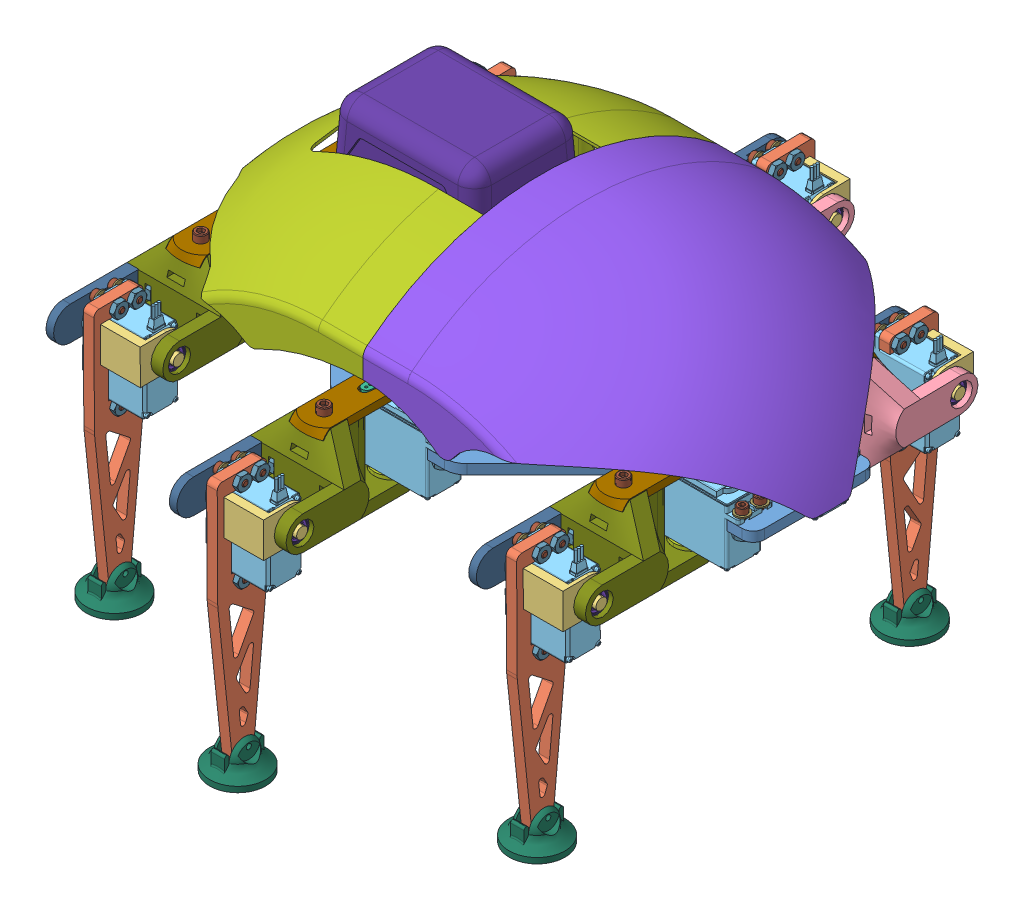
SolidWorks assembly Hexapod_NewBody, configuration Défaut. Lengths in mm. (continued)
Components (placement in the parent): (continued)
- Battery-1: Battery [Défaut] at (-118.1821 62.8376 15.5603) x (0 0 -1) z (-1 0 0) size (64.47 74.3 85.78)
  - MAKITA 4.0AH-1: MAKITA 4.0AH [Défaut] at (0.5853 -29.7874 85.4436) size (64.47 57.15 85.78)
  - MAKITA 4.0AH MOBILE-1: MAKITA 4.0AH MOBILE [Défaut] at (0.5853 -39.3124 91.7936) size (45.84 26.68 66.29)
- arduinoMega-1: arduinoMega [Detailed] at (-199.11 -7.6 14.62) x (0 0 -1) z (-1 0 0) size (108.32 14.5 53.3)
- raspberryPi3B-1: raspberryPi3B [Detailed] at (-109 6.35 15) x (-1 0 0) z (0 1 0) size (87.05 58.5 19.5)
- 12Channel PWM-1: 12Channel PWM [Default] at (-145.6 -5.6 15) x (-1 0 0) z (0 0 1) size (25.4 7.55 66.7)
- DROK_090483.stp-1: DROK_090483.stp [Default] at (-77.5 -5.6 45) x (-1 0 0) z (0 -1 0) size (50.02 60 18.9)
- socket head cap screw_ai-2: socket head cap screw_ai [HX-SHCS 0.138-32x0.625x0.625-N] at (-40.288 3.5052 19.09) x (0 -1 0) z (1 0 0) size (19.38 5.74 5.74)
- socket head cap screw_ai-3: socket head cap screw_ai [HX-SHCS 0.138-32x0.625x0.625-N] at (-50.288 3.5052 19.09) x (0 -1 0) z (0.5 0 0.866025) size (19.38 5.74 5.74)
- socket head cap screw_ai-4: socket head cap screw_ai [HX-SHCS 0.138-32x0.625x0.625-N] at (-50.288 3.5052 10.91) x (0 -1 0) z (1 0 0) size (19.38 5.74 5.74)
- socket head cap screw_ai-5: socket head cap screw_ai [HX-SHCS 0.138-32x0.625x0.625-N] at (-40.288 3.5052 10.91) x (0 -1 0) z (1 0 0) size (19.38 5.74 5.74)
- socket head cap screw_ai-6: socket head cap screw_ai [HX-SHCS 0.138-32x0.625x0.625-N] at (-170.288 3.5052 69.09) x (0 -1 0) z (1 0 0) size (19.38 5.74 5.74)
- socket head cap screw_ai-7: socket head cap screw_ai [HX-SHCS 0.138-32x0.625x0.625-N] at (-160.288 3.5052 69.09) x (0 -1 0) z (1 0 0) size (19.38 5.74 5.74)
- socket head cap screw_ai-14: socket head cap screw_ai [HX-SHCS 0.138-32x0.625x0.625-N] at (-160.288 3.5052 -39.09) x (0 -1 0) z (1 0 0) size (19.38 5.74 5.74)
- socket head cap screw_ai-15: socket head cap screw_ai [HX-SHCS 0.138-32x0.625x0.625-N] at (-170.288 3.5052 -39.09) x (0 -1 0) z (1 0 0) size (19.38 5.74 5.74)
- socket head cap screw_ai-16: socket head cap screw_ai [HX-SHCS 0.138-32x0.625x0.625-N] at (-280.288 3.5052 19.09) x (0 -1 0) z (1 0 0) size (19.38 5.74 5.74)
- socket head cap screw_ai-17: socket head cap screw_ai [HX-SHCS 0.138-32x0.625x0.625-N] at (-290.288 3.5052 19.09) x (0 -1 0) z (0.5 0 0.866025) size (19.38 5.74 5.74)
- socket head cap screw_ai-18: socket head cap screw_ai [HX-SHCS 0.138-32x0.625x0.625-N] at (-290.288 3.5052 10.91) x (0 -1 0) z (1 0 0) size (19.38 5.74 5.74)
- socket head cap screw_ai-19: socket head cap screw_ai [HX-SHCS 0.138-32x0.625x0.625-N] at (-280.288 3.5052 10.91) x (0 -1 0) z (1 0 0) size (19.38 5.74 5.74)
- machine screw nut hex_ai-60: machine screw nut hex_ai [MSHXNUT 0.138-32-D-N] at (-298.75 -8.4956 -15.08) x (1 0 0) z (0 -1 0) size (7.92 9.15 2.9)
- machine screw nut hex_ai-65: machine screw nut hex_ai [MSHXNUT 0.138-32-D-N] at (-298.75 -8.4956 -4.92) x (1 0 0) z (0 -1 0) size (7.92 9.15 2.9)
- machine screw nut hex_ai-70: machine screw nut hex_ai [MSHXNUT 0.138-32-D-N] at (-251.252 -8.4956 -4.92) x (0.5 0 0.866025) z (0 -1 0) size (7.92 9.15 2.9)
- machine screw nut hex_ai-75: machine screw nut hex_ai [MSHXNUT 0.138-32-D-N] at (-251.252 -8.4956 -15.08) x (0.5 0 0.866025) z (0 -1 0) size (7.92 9.15 2.9)
- machine screw nut hex_ai-80: machine screw nut hex_ai [MSHXNUT 0.138-32-D-N] at (-280.288 -13.5656 10.91) x (0 0 1) z (0 -1 0) size (7.92 9.15 2.9)
- machine screw nut hex_ai-85: machine screw nut hex_ai [MSHXNUT 0.138-32-D-N] at (-290.288 -13.5656 10.91) x (0 0 1) z (0 -1 0) size (7.92 9.15 2.9)
- machine screw nut hex_ai-63: machine screw nut hex_ai [MSHXNUT 0.138-32-D-N] at (-178.75 -8.4956 -65.08) x (1 0 0) z (0 -1 0) size (7.92 9.15 2.9)
- machine screw nut hex_ai-68: machine screw nut hex_ai [MSHXNUT 0.138-32-D-N] at (-178.75 -8.4956 -54.92) x (1 0 0) z (0 -1 0) size (7.92 9.15 2.9)
- machine screw nut hex_ai-73: machine screw nut hex_ai [MSHXNUT 0.138-32-D-N] at (-131.252 -8.4956 -54.92) x (0.5 0 0.866025) z (0 -1 0) size (7.92 9.15 2.9)
- machine screw nut hex_ai-78: machine screw nut hex_ai [MSHXNUT 0.138-32-D-N] at (-131.252 -8.4956 -65.08) x (0.5 0 0.866025) z (0 -1 0) size (7.92 9.15 2.9)
- machine screw nut hex_ai-83: machine screw nut hex_ai [MSHXNUT 0.138-32-D-N] at (-160.288 -13.5656 -39.09) x (0 0 1) z (0 -1 0) size (7.92 9.15 2.9)
- machine screw nut hex_ai-86: machine screw nut hex_ai [MSHXNUT 0.138-32-D-N] at (-170.288 -13.5656 -39.09) x (0 0 1) z (0 -1 0) size (7.92 9.15 2.9)
- machine screw nut hex_ai-87: machine screw nut hex_ai [MSHXNUT 0.138-32-D-N] at (-50.288 -13.5656 10.91) x (0 0 1) z (0 -1 0) size (7.92 9.15 2.9)
- machine screw nut hex_ai-84: machine screw nut hex_ai [MSHXNUT 0.138-32-D-N] at (-40.288 -13.5656 10.91) x (0 0 1) z (0 -1 0) size (7.92 9.15 2.9)
- machine screw nut hex_ai-74: machine screw nut hex_ai [MSHXNUT 0.138-32-D-N] at (-11.252 -8.4956 -4.92) x (0.5 0 0.866025) z (0 -1 0) size (7.92 9.15 2.9)
- machine screw nut hex_ai-79: machine screw nut hex_ai [MSHXNUT 0.138-32-D-N] at (-11.252 -8.4956 -15.08) x (0.5 0 0.866025) z (0 -1 0) size (7.92 9.15 2.9)
- machine screw nut hex_ai-69: machine screw nut hex_ai [MSHXNUT 0.138-32-D-N] at (-58.75 -8.4956 -4.92) x (1 0 0) z (0 -1 0) size (7.92 9.15 2.9)
- machine screw nut hex_ai-64: machine screw nut hex_ai [MSHXNUT 0.138-32-D-N] at (-58.75 -8.4956 -15.08) x (1 0 0) z (0 -1 0) size (7.92 9.15 2.9)
- machine screw nut hex_ai-88: machine screw nut hex_ai [MSHXNUT 0.138-32-D-N] at (-290.288 -10.67 19.09) x (0 0 -1) z (0 1 0) size (7.92 9.15 2.9)
- machine screw nut hex_ai-89: machine screw nut hex_ai [MSHXNUT 0.138-32-D-N] at (-280.288 -10.67 19.09) x (0 0 -1) z (0 1 0) size (7.92 9.15 2.9)
- machine screw nut hex_ai-90: machine screw nut hex_ai [MSHXNUT 0.138-32-D-N] at (-251.252 -5.6 34.92) x (0.5 0 -0.866025) z (0 1 0) size (7.92 9.15 2.9)
- machine screw nut hex_ai-91: machine screw nut hex_ai [MSHXNUT 0.138-32-D-N] at (-251.252 -5.6 45.08) x (0.5 0 -0.866025) z (0 1 0) size (7.92 9.15 2.9)
- machine screw nut hex_ai-92: machine screw nut hex_ai [MSHXNUT 0.138-32-D-N] at (-298.75 -5.6 34.92) x (1 0 0) z (0 1 0) size (7.92 9.15 2.9)
- machine screw nut hex_ai-93: machine screw nut hex_ai [MSHXNUT 0.138-32-D-N] at (-298.75 -5.6 45.08) x (1 0 0) z (0 1 0) size (7.92 9.15 2.9)
- machine screw nut hex_ai-94: machine screw nut hex_ai [MSHXNUT 0.138-32-D-N] at (-178.75 -5.6 95.08) x (1 0 0) z (0 1 0) size (7.92 9.15 2.9)
- machine screw nut hex_ai-95: machine screw nut hex_ai [MSHXNUT 0.138-32-D-N] at (-178.75 -5.6 84.92) x (1 0 0) z (0 1 0) size (7.92 9.15 2.9)
- machine screw nut hex_ai-96: machine screw nut hex_ai [MSHXNUT 0.138-32-D-N] at (-131.252 -5.6 84.92) x (0.5 0 -0.866025) z (0 1 0) size (7.92 9.15 2.9)
- machine screw nut hex_ai-97: machine screw nut hex_ai [MSHXNUT 0.138-32-D-N] at (-131.252 -5.6 95.08) x (0.5 0 -0.866025) z (0 1 0) size (7.92 9.15 2.9)
- machine screw nut hex_ai-98: machine screw nut hex_ai [MSHXNUT 0.138-32-D-N] at (-160.288 -10.67 69.09) x (0 0 -1) z (0 1 0) size (7.92 9.15 2.9)
- machine screw nut hex_ai-99: machine screw nut hex_ai [MSHXNUT 0.138-32-D-N] at (-170.288 -10.67 69.09) x (0 0 -1) z (0 1 0) size (7.92 9.15 2.9)
- machine screw nut hex_ai-100: machine screw nut hex_ai [MSHXNUT 0.138-32-D-N] at (-50.288 -10.67 19.09) x (0 0 -1) z (0 1 0) size (7.92 9.15 2.9)
- machine screw nut hex_ai-101: machine screw nut hex_ai [MSHXNUT 0.138-32-D-N] at (-40.288 -10.67 19.09) x (0 0 -1) z (0 1 0) size (7.92 9.15 2.9)
- machine screw nut hex_ai-102: machine screw nut hex_ai [MSHXNUT 0.138-32-D-N] at (-11.252 -5.6 34.92) x (0.5 0 -0.866025) z (0 1 0) size (7.92 9.15 2.9)
- machine screw nut hex_ai-103: machine screw nut hex_ai [MSHXNUT 0.138-32-D-N] at (-11.252 -5.6 45.08) x (0.5 0 -0.866025) z (0 1 0) size (7.92 9.15 2.9)
- machine screw nut hex_ai-104: machine screw nut hex_ai [MSHXNUT 0.138-32-D-N] at (-58.75 -5.6 34.92) x (1 0 0) z (0 1 0) size (7.92 9.15 2.9)
- machine screw nut hex_ai-105: machine screw nut hex_ai [MSHXNUT 0.138-32-D-N] at (-58.75 -5.6 45.08) x (1 0 0) z (0 1 0) size (7.92 9.15 2.9)
- socket head cap screw_ai-20: socket head cap screw_ai [HX-SHCS 0.138-32x0.5x0.5-N] at (-175 -12.6052 48.88) x (0 1 0) z (-0.5 0 -0.866025) size (16.21 5.74 5.74)
- socket head cap screw_ai-21: socket head cap screw_ai [HX-SHCS 0.138-32x0.5x0.5-N] at (-223.22 -12.6052 -32.36) x (0 1 0) z (1 0 0) size (16.21 5.74 5.74)
- socket head cap screw_ai-22: socket head cap screw_ai [HX-SHCS 0.138-32x0.5x0.5-N] at (-175 -12.6052 -26) x (0 1 0) z (-0.5 0 -0.866025) size (16.21 5.74 5.74)
- socket head cap screw_ai-23: socket head cap screw_ai [HX-SHCS 0.138-32x0.5x0.5-N] at (-223.22 -12.6052 50.11) x (0 1 0) z (-1 0 0) size (16.21 5.74 5.74)
- machine screw nut hex_ai-106: machine screw nut hex_ai [MSHXNUT 0.112-40-D-N] at (-223.22 2.4892 -32.36) x (1 0 0) z (0 1 0) size (6.35 7.33 2.49)
- machine screw nut hex_ai-107: machine screw nut hex_ai [MSHXNUT 0.112-40-D-N] at (-223.22 2.4892 50.11) x (1 0 0) z (0 1 0) size (6.35 7.33 2.49)
- machine screw nut hex_ai-108: machine screw nut hex_ai [MSHXNUT 0.112-40-D-N] at (-175 2.4892 -26) x (1 0 0) z (0 1 0) size (6.35 7.33 2.49)
- machine screw nut hex_ai-109: machine screw nut hex_ai [MSHXNUT 0.112-40-D-N] at (-175 2.4892 48.88) x (1 0 0) z (0 1 0) size (6.35 7.33 2.49)
- socket head cap screw_ai-24: socket head cap screw_ai [HX-SHCS 0.138-32x0.5x0.5-N] at (-117.315 -10.3052 -11.415) x (0 1 0) z (-0.5 0 -0.866025) size (16.21 5.74 5.74)
- machine screw nut hex_ai-110: machine screw nut hex_ai [MSHXNUT 0.112-40-D-N] at (-117.315 2.4892 -11.415) x (1 0 0) z (0 1 0) size (6.35 7.33 2.49)
- socket head cap screw_ai-25: socket head cap screw_ai [HX-SHCS 0.138-32x0.5x0.5-N] at (-80.685 -10.3052 -11.415) x (0 1 0) z (-0.5 0 -0.866025) size (16.21 5.74 5.74)
- socket head cap screw_ai-26: socket head cap screw_ai [HX-SHCS 0.138-32x0.5x0.5-N] at (-117.315 -10.3052 41.415) x (0 1 0) z (-0.5 0 -0.866025) size (16.21 5.74 5.74)
- socket head cap screw_ai-27: socket head cap screw_ai [HX-SHCS 0.138-32x0.5x0.5-N] at (-80.685 -10.3052 41.415) x (0 1 0) z (-0.5 0 -0.866025) size (16.21 5.74 5.74)
- machine screw nut hex_ai-111: machine screw nut hex_ai [MSHXNUT 0.112-40-D-N] at (-80.685 2.4892 -11.415) x (1 0 0) z (0 1 0) size (6.35 7.33 2.49)
- machine screw nut hex_ai-112: machine screw nut hex_ai [MSHXNUT 0.112-40-D-N] at (-117.315 2.4892 41.415) x (1 0 0) z (0 1 0) size (6.35 7.33 2.49)
- machine screw nut hex_ai-113: machine screw nut hex_ai [MSHXNUT 0.112-40-D-N] at (-80.685 2.4892 41.415) x (1 0 0) z (0 1 0) size (6.35 7.33 2.49)
- 1_4_Round_Aluminum_Standoff.step-1: 1_4_Round_Aluminum_Standoff.step [Défaut] at (-70 0 -9.5) x (0.963282 0 -0.268492) z (0.268492 0 0.963282) size (6.34 6.36 6.34)
- socket head cap screw_ai-28: socket head cap screw_ai [HX-SHCS 0.112-40x1x0.75-N] at (-70 10.4948 -9.5) x (0 -1 0) z (0.637638 0 0.770336) size (28.24 4.65 4.65)
- machine screw nut hex_ai-114: machine screw nut hex_ai [MSHXNUT 0.112-40-D-N] at (-70 -8.0892 -9.5) x (1 0 0) z (0 -1 0) size (6.35 7.33 2.49)
- 1_4_Round_Aluminum_Standoff.step-2: 1_4_Round_Aluminum_Standoff.step [Défaut] at (-128 0 -9.5) x (0.963282 0 -0.268492) z (0.268492 0 0.963282) size (6.34 6.36 6.34)
- 1_4_Round_Aluminum_Standoff.step-3: 1_4_Round_Aluminum_Standoff.step [Défaut] at (-70 0 39.5) x (0.963282 0 -0.268492) z (0.268492 0 0.963282) size (6.34 6.36 6.34)
- 1_4_Round_Aluminum_Standoff.step-4: 1_4_Round_Aluminum_Standoff.step [Défaut] at (-128 0 39.5) x (0.963282 0 -0.268492) z (0.268492 0 0.963282) size (6.34 6.36 6.34)
- machine screw nut hex_ai-115: machine screw nut hex_ai [MSHXNUT 0.112-40-D-N] at (-128 -8.0892 -9.5) x (1 0 0) z (0 -1 0) size (6.35 7.33 2.49)
- machine screw nut hex_ai-116: machine screw nut hex_ai [MSHXNUT 0.112-40-D-N] at (-70 -8.0892 39.5) x (1 0 0) z (0 -1 0) size (6.35 7.33 2.49)
- machine screw nut hex_ai-117: machine screw nut hex_ai [MSHXNUT 0.112-40-D-N] at (-128 -8.0892 39.5) x (1 0 0) z (0 -1 0) size (6.35 7.33 2.49)
- socket head cap screw_ai-29: socket head cap screw_ai [HX-SHCS 0.112-40x1x0.75-N] at (-128 10.4948 -9.5) x (0 -1 0) z (0.637638 0 0.770336) size (28.24 4.65 4.65)
- socket head cap screw_ai-30: socket head cap screw_ai [HX-SHCS 0.112-40x1x0.75-N] at (-70 10.4948 39.5) x (0 -1 0) z (0.637638 0 0.770336) size (28.24 4.65 4.65)
- socket head cap screw_ai-31: socket head cap screw_ai [HX-SHCS 0.112-40x1x0.75-N] at (-128 10.4948 39.5) x (0 -1 0) z (0.637638 0 0.770336) size (28.24 4.65 4.65)
- socket head cap screw_ai-32: socket head cap screw_ai [HX-SHCS 0.112-40x0.5x0.5-N] at (-155 -9.9448 -12.95) x (0 1 0) z (-1 0 0) size (15.54 4.65 4.65)
- machine screw nut hex_ai-118: machine screw nut hex_ai [MSHXNUT 0.112-40-D-N] at (-155 2.4892 -12.95) x (1 0 0) z (0 1 0) size (6.35 7.33 2.49)
- socket head cap screw_ai-33: socket head cap screw_ai [HX-SHCS 0.112-40x0.5x0.5-N] at (-136.2 -9.9448 -12.95) x (0 1 0) z (-1 0 0) size (15.54 4.65 4.65)
- socket head cap screw_ai-34: socket head cap screw_ai [HX-SHCS 0.112-40x0.5x0.5-N] at (-155 -9.9448 42.95) x (0 1 0) z (-1 0 0) size (15.54 4.65 4.65)
- socket head cap screw_ai-35: socket head cap screw_ai [HX-SHCS 0.112-40x0.5x0.5-N] at (-136.2 -9.9448 42.95) x (0 1 0) z (-1 0 0) size (15.54 4.65 4.65)
- machine screw nut hex_ai-119: machine screw nut hex_ai [MSHXNUT 0.112-40-D-N] at (-136.2 2.4892 -12.95) x (1 0 0) z (0 1 0) size (6.35 7.33 2.49)
- machine screw nut hex_ai-120: machine screw nut hex_ai [MSHXNUT 0.112-40-D-N] at (-155 2.4892 42.95) x (1 0 0) z (0 1 0) size (6.35 7.33 2.49)
- machine screw nut hex_ai-121: machine screw nut hex_ai [MSHXNUT 0.112-40-D-N] at (-136.2 2.4892 42.95) x (1 0 0) z (0 1 0) size (6.35 7.33 2.49)
- 1_4_Round_Aluminum_Standoff.step-5: 1_4_Round_Aluminum_Standoff.step [Défaut] at (-174 0 -7) x (0.963282 0 -0.268492) z (0.268492 0 0.963282) size (6.34 6.36 6.34)
- 1_4_Round_Aluminum_Standoff.step-6: 1_4_Round_Aluminum_Standoff.step [Défaut] at (-174 0 37) x (0.963282 0 -0.268492) z (0.268492 0 0.963282) size (6.34 6.36 6.34)
- 1_4_Round_Aluminum_Standoff.step-7: 1_4_Round_Aluminum_Standoff.step [Défaut] at (-240 0 -7) x (0.963282 0 -0.268492) z (0.268492 0 0.963282) size (6.34 6.36 6.34)
- 1_4_Round_Aluminum_Standoff.step-8: 1_4_Round_Aluminum_Standoff.step [Défaut] at (-240 0 37) x (0.963282 0 -0.268492) z (0.268492 0 0.963282) size (6.34 6.36 6.34)
- socket head cap screw_ai-40: socket head cap screw_ai [HX-SHCS 0.112-40x1x0.75-N] at (-174 -8.4448 -7) x (0 1 0) z (-0.415316 0 -0.909677) size (28.24 4.65 4.65)
- socket head cap screw_ai-41: socket head cap screw_ai [HX-SHCS 0.112-40x1x0.75-N] at (-174 -8.4448 37) x (0 1 0) z (-0.415316 0 -0.909677) size (28.24 4.65 4.65)
- socket head cap screw_ai-42: socket head cap screw_ai [HX-SHCS 0.112-40x1x0.75-N] at (-240 -8.4448 -7) x (0 1 0) z (-0.415316 0 -0.909677) size (28.24 4.65 4.65)
- socket head cap screw_ai-43: socket head cap screw_ai [HX-SHCS 0.112-40x1x0.75-N] at (-240 -8.4448 37) x (0 1 0) z (-0.415316 0 -0.909677) size (28.24 4.65 4.65)
- Batterie_holder-1: Batterie_holder [Default] at (-223 17.7 15) size (72 19.6 50)
- machine screw nut hex_ai-122: machine screw nut hex_ai [MSHXNUT 0.112-40-D-N] at (-174 15.1892 -7) x (1 0 0) z (0 1 0) size (6.35 7.33 2.49)
- machine screw nut hex_ai-123: machine screw nut hex_ai [MSHXNUT 0.112-40-D-N] at (-174 15.1892 37) x (1 0 0) z (0 1 0) size (6.35 7.33 2.49)
- machine screw nut hex_ai-124: machine screw nut hex_ai [MSHXNUT 0.112-40-D-N] at (-240 15.1892 -7) x (1 0 0) z (0 1 0) size (6.35 7.33 2.49)
- machine screw nut hex_ai-125: machine screw nut hex_ai [MSHXNUT 0.112-40-D-N] at (-240 15.1892 37) x (1 0 0) z (0 1 0) size (6.35 7.33 2.49)
- Shell_front-3: Shell_front [Default] at (-155 -76.2 15) x (0 0 1) z (-1 0 0) size (204.71 79.03 165.14)
- Shell_back-3: Shell_back [Default] at (-155 -76.2 15) x (0 0 -1) z (1 0 0) size (205.09 91.22 173.55)
Mates (geometry in assembly coordinates):
- Coincident2: coincident anti-aligned: plane of Body_V2-5 through (-295 -5.601 0) normal (0 0 -1)
- Coincident3: coincident aligned: plane of Body_V2-5 through (-310 0 15) normal (0 1 0)
- Coincident4: coincident aligned: plane of Body_V2-5 through (0 0 50) normal (1 0 0)
- Coincident5: coincident anti-aligned: plane of Body_V2-5 through (-310 0 15) normal (0 1 0); plane of Leg-6/hs-422-3 through (-35.001 0 -0.094) normal (0 -1 0)
- Concentric3: concentric anti-aligned: cylinder of Body_V2-5 through (-58.75 0 -15.08) axis (0 -1 0) radius 1.45; cylinder of Leg-6/hs-422-3 through (-58.75 -26.67 -15.08) axis (0 1 0) radius 2.1844
- Concentric6: concentric aligned: cylinder of Body_V2-5 through (-298.75 -5.601 -4.92) axis (0 1 0) radius 1.45; cylinder of Leg-7/hs-422-3 through (-298.75 -26.67 -4.92) axis (0 1 0) radius 2.1844
- Parallel4: parallel anti-aligned: plane of Body_V2-5 through (-295 -5.601 0) normal (0 0 -1); plane of Leg-7/hs-422-3 through (-275.001 -5.969 -0.094) normal (0 0 1)
- Coincident9: coincident anti-aligned: plane of Body_V2-5 through (-310 0 15) normal (0 1 0); plane of Leg-7/hs-422-3 through (-275.001 0 -0.094) normal (0 -1 0)
- Coincident10: coincident anti-aligned: plane of Body_V2-5 through (-310 0 15) normal (0 1 0); plane of Leg-8/hs-422-3 through (-155.001 0 -50.094) normal (0 -1 0)
- Concentric7: concentric anti-aligned: cylinder of Body_V2-5 through (-178.75 0 -54.92) axis (0 -1 0) radius 1.45; cylinder of Leg-8/hs-422-3 through (-178.75 -26.67 -54.92) axis (0 1 0) radius 2.1844
- Parallel5: parallel anti-aligned: plane of Body_V2-5 through (-175 -5.6 -50) normal (0 0 -1); plane of Leg-8/hs-422-3 through (-155.001 -5.969 -50.094) normal (0 0 1)
- Parallel6: parallel anti-aligned: plane of Body_V2-5 through (-55 -5.6 0) normal (0 0 -1); plane of Leg-6/hs-422-3 through (-35.001 -5.969 -0.094) normal (0 0 1)
- Coincident11: coincident anti-aligned: plane of Body_V2-5 through (-310 0 15) normal (0 1 0); plane of Leg_(Straight_Foot)_(Mirror)-4/hs-422-3 through (-275.001 0 49.906) normal (0 -1 0)
- Concentric8: concentric aligned: cylinder of Body_V2-5 through (-298.75 -5.601 45.08) axis (0 1 0) radius 1.45; cylinder of Leg_(Straight_Foot)_(Mirror)-4/hs-422-3 through (-298.75 -26.67 45.08) axis (0 1 0) radius 2.1844
- Parallel7: parallel anti-aligned: plane of Body_V2-5 through (-295 -5.601 30) normal (0 0 1); plane of Leg_(Straight_Foot)_(Mirror)-4/hs-422-3 through (-275.001 -5.969 30.094) normal (0 0 -1)
- Coincident13: coincident anti-aligned: plane of Body_V2-5 through (-310 0 15) normal (0 1 0); plane of Leg_(Straight_Foot)_(Mirror)-5/hs-422-3 through (-35.001 0 49.906) normal (0 -1 0)
- Concentric9: concentric anti-aligned: cylinder of Body_V2-5 through (-58.75 0 45.08) axis (0 -1 0) radius 1.45; cylinder of Leg_(Straight_Foot)_(Mirror)-5/hs-422-3 through (-58.75 -26.67 45.08) axis (0 1 0) radius 2.1844
- Parallel8: parallel anti-aligned: plane of Body_V2-5 through (-55 -5.6 30) normal (0 0 1); plane of Leg_(Straight_Foot)_(Mirror)-5/hs-422-3 through (-35.001 -5.969 30.094) normal (0 0 -1)
- Coincident15: coincident anti-aligned: plane of Body_V2-5 through (-310 0 15) normal (0 1 0); plane of Leg_(Straight_Foot)_(Mirror)-6/hs-422-3 through (-155.001 0 99.906) normal (0 -1 0)
- Concentric10: concentric anti-aligned: cylinder of Body_V2-5 through (-178.75 0 95.08) axis (0 -1 0) radius 1.45; cylinder of Leg_(Straight_Foot)_(Mirror)-6/hs-422-3 through (-178.75 -26.67 95.08) axis (0 1 0) radius 2.1844
- Parallel9: parallel anti-aligned: plane of Body_V2-5 through (-175 -5.6 80) normal (0 0 1); plane of Leg_(Straight_Foot)_(Mirror)-6/hs-422-3 through (-155.001 -5.969 80.094) normal (0 0 -1)
- Coïncidente2: coincident anti-aligned: plane of arduinoMega-1 through (-199.11 -5.6 14.62) normal (0 1 0); plane of Body_V2-5 through (-310 -5.6 15) normal (0 -1 0)
- Coïncidente4: coincident anti-aligned: plane of Body_V2-5 through (-310 -5.6 15) normal (0 -1 0); plane of 12Channel PWM-1 through (-155 -5.6 -12.95) normal (0 1 0)
- Coïncidente5: coincident anti-aligned: plane of Body_V2-5 through (-310 -5.6 15) normal (0 -1 0); plane of DROK_090483.stp-1 through (-99 -5.6 15) normal (0 1 0)
- Parallèle4: parallel aligned: plane of Body_V2-5 through (0 0 50) normal (1 0 0); plane of 12Channel PWM-1 through (-132.9 -7.1 -12.95) normal (1 0 0)
- Concentric13: concentric aligned: cylinder of Body_V2-5 through (-155 0 42.95) axis (0 -1 0) radius 1.25; cylinder of 12Channel PWM-1 through (-155 -2.0645 42.95) axis (0 -1 0) radius 1.25
- Concentric17: concentric anti-aligned: circle of Body-1; circle of DROK_090483.stp-1
- Concentric18: concentric aligned: cylinder of Body_V2-5 through (-80.685 0 41.415) axis (0 -1 0) radius 1.45; cylinder of DROK_090483.stp-1 through (-80.685 -5.6 41.415) axis (0 -1 0) radius 1.585
- Concentric19: concentric aligned: cylinder of Body_V2-5 through (-175 0 -26) axis (0 -1 0) radius 1.6; circle of arduinoMega-1
- Concentric22: concentric aligned: cylinder of Body_V2-5 through (-223.22 0 50.11) axis (0 -1 0) radius 1.6; cylinder of arduinoMega-1 through (-223.22 -7.6 50.11) axis (0 -1 0) radius 1.6
- Concentric23: concentric anti-aligned: cylinder of Body_V2-5 through (-40.288 0 19.09) axis (0 -1 0) radius 1.45; cylinder of socket head cap screw_ai-2 through (-40.288 35.2552 19.09) axis (0 1 0) radius 1.7526
- Concentric24: concentric anti-aligned: cylinder of Body_V2-5 through (-50.288 0 19.09) axis (0 -1 0) radius 1.45; cylinder of socket head cap screw_ai-3 through (-50.288 35.2552 19.09) axis (0 1 0) radius 1.7526
- Coincident19: coincident anti-aligned: plane of Body_V2-5 through (-310 0 15) normal (0 1 0); plane of socket head cap screw_ai-2 through (-40.288 0 16.2198) normal (0 -1 0)
- Coincident20: coincident anti-aligned: plane of Body_V2-5 through (-310 0 15) normal (0 1 0); plane of socket head cap screw_ai-3 through (-47.8023 0 17.6549) normal (0 -1 0)
- Parallel10: parallel aligned: plane of Body_V2-5 through (0 0 50) normal (1 0 0); plane of socket head cap screw_ai-3 through (-51.6723 1.8796 19.8892) normal (1 0 0)
- Parallel11: parallel aligned: plane of Body_V2-5 through (0 0 50) normal (1 0 0); plane of socket head cap screw_ai-2 through (-41.6723 1.8796 18.2908) normal (1 0 0)
- Concentric25: concentric anti-aligned: cylinder of Body_V2-5 through (-50.288 0 10.91) axis (0 -1 0) radius 1.45; cylinder of socket head cap screw_ai-4 through (-50.288 35.2552 10.91) axis (0 1 0) radius 1.7526
- Concentric26: concentric anti-aligned: cylinder of Body_V2-5 through (-40.288 0 10.91) axis (0 -1 0) radius 1.45; cylinder of socket head cap screw_ai-5 through (-40.288 35.2552 10.91) axis (0 1 0) radius 1.7526
- Coincident23: coincident anti-aligned: plane of Body_V2-5 through (-310 0 15) normal (0 1 0); plane of socket head cap screw_ai-5 through (-40.288 0 8.0398) normal (0 -1 0)
- Coincident24: coincident anti-aligned: plane of Body_V2-5 through (-310 0 15) normal (0 1 0); plane of socket head cap screw_ai-4 through (-50.288 0 8.0398) normal (0 -1 0)
- Parallel12: parallel aligned: plane of Body_V2-5 through (0 0 50) normal (1 0 0); plane of socket head cap screw_ai-5 through (-41.6723 1.8796 10.1108) normal (1 0 0)
- Parallel13: parallel aligned: plane of Body_V2-5 through (0 0 50) normal (1 0 0); plane of socket head cap screw_ai-4 through (-51.6723 1.8796 10.1108) normal (1 0 0)
- Concentric27: concentric anti-aligned: cylinder of Body_V2-5 through (-170.288 0 -39.09) axis (0 -1 0) radius 1.45; cylinder of HX-SHCS 0.138-32x0.625x0.625-N-13 through (-214.94 40.2807 -39.09) axis (0 1 0) radius 1.7526
- Concentric29: concentric anti-aligned: cylinder of Body_V2-5 through (-160.288 0 69.09) axis (0 -1 0) radius 1.45; cylinder of socket head cap screw_ai-7 through (-160.288 35.2552 69.09) axis (0 1 0) radius 1.7526
- Concentric30: concentric anti-aligned: cylinder of Body_V2-5 through (-170.288 0 69.09) axis (0 -1 0) radius 1.45; cylinder of socket head cap screw_ai-6 through (-170.288 35.2552 69.09) axis (0 1 0) radius 1.7526
- Coincident27: coincident anti-aligned: plane of Body_V2-5 through (-310 0 15) normal (0 1 0); plane of socket head cap screw_ai-7 through (-160.288 0 66.2198) normal (0 -1 0)
- Coincident28: coincident anti-aligned: plane of Body_V2-5 through (-310 0 15) normal (0 1 0); plane of socket head cap screw_ai-6 through (-170.288 0 66.2198) normal (0 -1 0)
- Parallel14: parallel aligned: plane of Body_V2-5 through (0 0 50) normal (1 0 0); plane of socket head cap screw_ai-6 through (-171.6723 1.8796 68.2908) normal (1 0 0)
- Parallel15: parallel aligned: plane of Body_V2-5 through (0 0 50) normal (1 0 0); plane of socket head cap screw_ai-7 through (-161.6723 1.8796 68.2908) normal (1 0 0)
- Concentric31: concentric anti-aligned: cylinder of Body_V2-5 through (-170.288 0 -39.09) axis (0 -1 0) radius 1.45; cylinder of socket head cap screw_ai-15 through (-170.288 35.2552 -39.09) axis (0 1 0) radius 1.7526
- Concentric32: concentric anti-aligned: cylinder of Body_V2-5 through (-160.288 0 -39.09) axis (0 -1 0) radius 1.45; cylinder of socket head cap screw_ai-14 through (-160.288 35.2552 -39.09) axis (0 1 0) radius 1.7526
- Coincident31: coincident anti-aligned: plane of Body_V2-5 through (-310 0 15) normal (0 1 0); plane of socket head cap screw_ai-15 through (-170.288 0 -41.9602) normal (0 -1 0)
- Coincident32: coincident anti-aligned: plane of Body_V2-5 through (-310 0 15) normal (0 1 0); plane of socket head cap screw_ai-14 through (-160.288 0 -41.9602) normal (0 -1 0)
- Parallel16: parallel anti-aligned: plane of Body_V2-5 through (0 0 50) normal (1 0 0); plane of socket head cap screw_ai-15 through (-168.9037 1.8796 -38.2908) normal (-1 0 0)
- Parallel17: parallel anti-aligned: plane of Body_V2-5 through (0 0 50) normal (1 0 0); plane of socket head cap screw_ai-14 through (-158.9037 1.8796 -38.2908) normal (-1 0 0)
- Concentric33: concentric aligned: cylinder of Body_V2-5 through (-290.288 -5.601 19.09) axis (0 1 0) radius 1.45; cylinder of socket head cap screw_ai-17 through (-290.288 35.2552 19.09) axis (0 1 0) radius 1.7526
- Concentric34: concentric aligned: circle of Body-1; cylinder of socket head cap screw_ai-16 through (-280.288 35.2552 19.09) axis (0 1 0) radius 1.7526
- Concentric35: concentric aligned: cylinder of Body_V2-5 through (-290.288 -5.601 10.91) axis (0 1 0) radius 1.45; cylinder of socket head cap screw_ai-18 through (-290.288 35.2552 10.91) axis (0 1 0) radius 1.7526
- Concentric36: concentric aligned: cylinder of Body_V2-5 through (-280.288 -5.601 10.91) axis (0 1 0) radius 1.45; cylinder of socket head cap screw_ai-19 through (-280.288 35.2552 10.91) axis (0 1 0) radius 1.7526
- Coincident35: coincident anti-aligned: plane of Body_V2-5 through (-310 0 15) normal (0 1 0); plane of socket head cap screw_ai-18 through (-290.288 0 8.0398) normal (0 -1 0)
- Coincident36: coincident anti-aligned: plane of Body_V2-5 through (-310 0 15) normal (0 1 0); plane of socket head cap screw_ai-19 through (-280.288 0 8.0398) normal (0 -1 0)
- Coincident37: coincident anti-aligned: plane of Body_V2-5 through (-310 0 15) normal (0 1 0); plane of socket head cap screw_ai-17 through (-287.8023 0 17.6549) normal (0 -1 0)
- Coincident38: coincident anti-aligned: plane of Body_V2-5 through (-310 0 15) normal (0 1 0); plane of socket head cap screw_ai-16 through (-280.288 0 16.2198) normal (0 -1 0)
- Parallel18: parallel anti-aligned: plane of Body_V2-5 through (0 0 50) normal (1 0 0); plane of socket head cap screw_ai-19 through (-278.9037 1.8796 11.7092) normal (-1 0 0)
- Parallel19: parallel anti-aligned: plane of Body_V2-5 through (0 0 50) normal (1 0 0); plane of socket head cap screw_ai-18 through (-288.9037 1.8796 11.7092) normal (-1 0 0)
- Parallel20: parallel anti-aligned: plane of Body_V2-5 through (0 0 50) normal (1 0 0); plane of socket head cap screw_ai-16 through (-278.9037 1.8796 19.8892) normal (-1 0 0)
- Parallel21: parallel anti-aligned: plane of Body_V2-5 through (0 0 50) normal (1 0 0); plane of socket head cap screw_ai-17 through (-288.9037 1.8796 18.2908) normal (-1 0 0)
- Concentric37: concentric anti-aligned: cylinder of Leg-7/socket_1_2_6-32_with_washer-7/socket head cap screw_ai-1 through (-298.75 38.5826 -15.08) axis (0 1 0) radius 1.7526; circle of MSHXNUT 0.138-32-D-N-1
- Coincident40: coincident anti-aligned: plane of Body_V2-5 through (-310 -5.6 15) normal (0 -1 0); plane of machine screw nut hex_ai-60 through (-298.75 -5.6 -10.5046) normal (0 1 0)
- Parallel22: parallel aligned: plane of Leg-7/hs-422-3 through (-294.94 -5.969 -0.094) normal (-1 0 0); plane of machine screw nut hex_ai-60 through (-302.7124 -5.6 -12.7923) normal (-1 0 0)
- Concentric38: concentric anti-aligned: cylinder of Leg-7/socket_1_2_6-32_with_washer-5/socket head cap screw_ai-1 through (-298.75 38.5826 -4.92) axis (0 1 0) radius 1.7526; circle of MSHXNUT 0.138-32-D-N-2
- Parallel23: parallel aligned: plane of Leg-7/hs-422-3 through (-294.94 -5.969 -0.094) normal (-1 0 0); plane of machine screw nut hex_ai-65 through (-302.7124 -5.6 -2.6323) normal (-1 0 0)
- Coincident44: coincident anti-aligned: plane of Body_V2-5 through (-310 -5.6 15) normal (0 -1 0); plane of machine screw nut hex_ai-65 through (-298.75 -5.6 -0.3446) normal (0 1 0)
- Coincident45: coincident anti-aligned: cylinder of Leg-7/socket_1_2_6-32_with_washer-8/socket head cap screw_ai-1 through (-251.252 38.5826 -4.92) axis (0 1 0) radius 1.7526; circle of MSHXNUT 0.138-32-D-N-3
- Concentric40: concentric anti-aligned: cylinder of Leg-7/socket_1_2_6-32_with_washer-6/socket head cap screw_ai-1 through (-251.252 38.5826 -15.08) axis (0 1 0) radius 1.7526; circle of MSHXNUT 0.138-32-D-N-4
- Coincident47: coincident anti-aligned: plane of Body_V2-5 through (-310 -5.6 15) normal (0 -1 0); plane of machine screw nut hex_ai-75 through (-255.2144 -5.6 -12.7923) normal (0 1 0)
- Coincident48: coincident anti-aligned: plane of Body_V2-5 through (-310 -5.6 15) normal (0 -1 0); plane of machine screw nut hex_ai-70 through (-255.2144 -5.6 -2.6323) normal (0 1 0)
- Parallel24: parallel aligned: plane of Leg-7/hs-422-3 through (-255.062 -5.969 -0.094) normal (1 0 0); plane of machine screw nut hex_ai-75 through (-247.2896 -5.6 -17.3677) normal (1 0 0)
- Parallel25: parallel aligned: plane of Leg-7/hs-422-3 through (-255.062 -5.969 -0.094) normal (1 0 0); plane of machine screw nut hex_ai-70 through (-247.2896 -5.6 -7.2077) normal (1 0 0)
- Concentric41: concentric anti-aligned: cylinder of socket head cap screw_ai-19 through (-280.288 35.2552 10.91) axis (0 1 0) radius 1.7526; circle of MSHXNUT 0.138-32-D-N-5
- Concentric42: concentric anti-aligned: cylinder of socket head cap screw_ai-18 through (-290.288 35.2552 10.91) axis (0 1 0) radius 1.7526; circle of MSHXNUT 0.138-32-D-N-6
- Coincident53: coincident anti-aligned: plane of Leg-7/Bearing_mount_leg-1 through (-295.288 -10.67 15) normal (0 -1 0); plane of machine screw nut hex_ai-85 through (-294.8634 -10.67 10.91) normal (0 1 0)
- Coincident54: coincident anti-aligned: plane of Leg-7/Bearing_mount_leg-1 through (-295.288 -10.67 15) normal (0 -1 0); plane of machine screw nut hex_ai-80 through (-284.8634 -10.67 10.91) normal (0 1 0)
- Parallel26: parallel aligned: plane of Leg-7/Bearing_mount_leg-1 through (-295.288 -26.67 5) normal (0 0 1); plane of machine screw nut hex_ai-80 through (-282.5757 -10.67 14.8724) normal (0 0 1)
- Parallel27: parallel aligned: plane of Leg-7/Bearing_mount_leg-1 through (-295.288 -26.67 5) normal (0 0 1); plane of machine screw nut hex_ai-85 through (-292.5757 -10.67 14.8724) normal (0 0 1)
- Concentric43: concentric aligned: cylinder of arduinoMega-1 through (-175 -7.6 48.88) axis (0 -1 0) radius 1.6; cylinder of socket head cap screw_ai-20 through (-175 -44.3552 48.88) axis (0 -1 0) radius 1.7526
- Concentric44: concentric aligned: cylinder of arduinoMega-1 through (-223.22 -7.6 50.11) axis (0 -1 0) radius 1.6; cylinder of socket head cap screw_ai-23 through (-223.22 -44.3552 50.11) axis (0 -1 0) radius 1.7526
- Concentric45: concentric aligned: cylinder of arduinoMega-1 through (-223.22 -7.6 -32.36) axis (0 -1 0) radius 1.6; cylinder of socket head cap screw_ai-21 through (-223.22 -44.3552 -32.36) axis (0 -1 0) radius 1.7526
- Concentric46: concentric aligned: cylinder of arduinoMega-1 through (-175 -7.6 -26) axis (0 -1 0) radius 1.6; cylinder of socket head cap screw_ai-22 through (-175 -44.3552 -26) axis (0 -1 0) radius 1.7526
- Coincident58: coincident anti-aligned: plane of arduinoMega-1 through (-199.11 -9.1 14.62) normal (0 -1 0); plane of socket head cap screw_ai-20 through (-172.5143 -9.1 47.4449) normal (0 1 0)
- Coincident59: coincident anti-aligned: plane of arduinoMega-1 through (-199.11 -9.1 14.62) normal (0 -1 0); plane of socket head cap screw_ai-22 through (-172.5143 -9.1 -27.4351) normal (0 1 0)
- Coincident60: coincident anti-aligned: plane of arduinoMega-1 through (-199.11 -9.1 14.62) normal (0 -1 0); plane of socket head cap screw_ai-23 through (-223.22 -9.1 47.2398) normal (0 1 0)
- Coincident61: coincident anti-aligned: plane of arduinoMega-1 through (-199.11 -9.1 14.62) normal (0 -1 0); plane of socket head cap screw_ai-21 through (-223.22 -9.1 -29.4898) normal (0 1 0)
- Concentric47: concentric anti-aligned: cylinder of socket head cap screw_ai-21 through (-223.22 -44.3552 -32.36) axis (0 -1 0) radius 1.7526; circle of MSHXNUT 0.112-40-S-N-2
- Concentric48: concentric anti-aligned: cylinder of socket head cap screw_ai-23 through (-223.22 -44.3552 50.11) axis (0 -1 0) radius 1.7526; circle of MSHXNUT 0.112-40-S-N-3
- Concentric49: concentric anti-aligned: cylinder of socket head cap screw_ai-22 through (-175 -44.3552 -26) axis (0 -1 0) radius 1.7526; circle of MSHXNUT 0.112-40-S-N-4
- Concentric50: concentric anti-aligned: cylinder of socket head cap screw_ai-20 through (-175 -44.3552 48.88) axis (0 -1 0) radius 1.7526; circle of MSHXNUT 0.112-40-S-N-5
- Coincident62: coincident anti-aligned: plane of Body_V2-5 through (-310 0 15) normal (0 1 0); plane of machine screw nut hex_ai-109 through (-181.35 0 48.88) normal (0 -1 0)
- Coincident63: coincident anti-aligned: plane of Body_V2-5 through (-310 0 15) normal (0 1 0); plane of machine screw nut hex_ai-108 through (-181.35 0 -26) normal (0 -1 0)
- Coincident64: coincident anti-aligned: plane of Body_V2-5 through (-310 0 15) normal (0 1 0); plane of machine screw nut hex_ai-107 through (-229.57 0 50.11) normal (0 -1 0)
- Coincident65: coincident anti-aligned: plane of Body_V2-5 through (-310 0 15) normal (0 1 0); plane of machine screw nut hex_ai-106 through (-229.57 0 -32.36) normal (0 -1 0)
- Parallel28: parallel anti-aligned: plane of Body_V2-5 through (-310 0 15) normal (-1 0 0); plane of machine screw nut hex_ai-107 through (-220.045 0 48.2769) normal (1 0 0)
- Parallel30: parallel aligned: plane of Body_V2-5 through (-310 0 15) normal (-1 0 0); plane of machine screw nut hex_ai-106 through (-226.395 0 -34.1931) normal (-1 0 0)
- Parallel31: parallel aligned: plane of Body_V2-5 through (-310 0 15) normal (-1 0 0); plane of machine screw nut hex_ai-108 through (-178.175 0 -27.8331) normal (-1 0 0)
- Parallel32: parallel aligned: plane of Body_V2-5 through (-310 0 15) normal (-1 0 0); plane of machine screw nut hex_ai-109 through (-178.175 0 47.0469) normal (-1 0 0)
- Parallel33: parallel aligned: plane of arduinoMega-1 through (-225.76 -9.1 64.11) normal (-1 0 0); plane of socket head cap screw_ai-23 through (-221.8357 -10.9796 49.3108) normal (-1 0 0)
- Parallel34: parallel aligned: plane of arduinoMega-1 through (-225.76 -9.1 64.11) normal (-1 0 0); plane of socket head cap screw_ai-20 through (-173.6157 -10.9796 48.0808) normal (-1 0 0)
- Parallel35: parallel aligned: plane of arduinoMega-1 through (-225.76 -9.1 64.11) normal (-1 0 0); plane of socket head cap screw_ai-22 through (-173.6157 -10.9796 -26.7992) normal (-1 0 0)
- Parallel36: parallel aligned: plane of arduinoMega-1 through (-225.76 -9.1 64.11) normal (-1 0 0); plane of socket head cap screw_ai-21 through (-221.8357 -10.9796 -33.1592) normal (-1 0 0)
- Concentric51: concentric aligned: cylinder of DROK_090483.stp-1 through (-117.315 -5.6 -11.415) axis (0 -1 0) radius 1.585; cylinder of socket head cap screw_ai-24 through (-117.315 -42.0552 -11.415) axis (0 -1 0) radius 1.7526
- Coincident74: coincident anti-aligned: plane of DROK_090483.stp-1 through (-99 -6.8 15) normal (0 -1 0); plane of socket head cap screw_ai-24 through (-114.8293 -6.8 -12.8501) normal (0 1 0)
- Parallel37: parallel aligned: plane of DROK_090483.stp-1 through (-120.5 -5.6 45) normal (-1 0 0); plane of socket head cap screw_ai-24 through (-115.9307 -8.6796 -12.2142) normal (-1 0 0)
- Concentric52: concentric anti-aligned: cylinder of socket head cap screw_ai-24 through (-117.315 -42.0552 -11.415) axis (0 -1 0) radius 1.7526; circle of MSHXNUT 0.112-40-S-N-6
- Coincident76: coincident anti-aligned: plane of Body_V2-5 through (-310 0 15) normal (0 1 0); plane of machine screw nut hex_ai-110 through (-123.665 0 -11.415) normal (0 -1 0)
- Parallel38: parallel anti-aligned: plane of Body_V2-5 through (0 0 50) normal (1 0 0); plane of machine screw nut hex_ai-110 through (-120.49 0 -13.2481) normal (-1 0 0)
- Concentric53: concentric anti-aligned: cylinder of Body_V2-5 through (-70 -5.6 -9.5) axis (0 1 0) radius 1.375; cylinder of 1_4_Round_Aluminum_Standoff.step-1 through (-70 6.35 -9.5) axis (0 -1 0) radius 3.1712
- Coincident78: coincident anti-aligned: plane of Body_V2-5 through (-310 0 15) normal (0 1 0); plane of 1_4_Round_Aluminum_Standoff.step-1 through (-70 0 -9.5) normal (0 -1 0)
- Coincident83: coincident anti-aligned: plane of Body_V2-5 through (-310 -5.6 15) normal (0 -1 0); plane of machine screw nut hex_ai-114 through (-76.35 -5.6 -9.5) normal (0 1 0)
- Parallel40: parallel aligned: plane of Body_V2-5 through (0 0 50) normal (1 0 0); plane of machine screw nut hex_ai-114 through (-66.825 -5.6 -7.6669) normal (1 0 0)
- Concentric56: concentric aligned: cylinder of 12Channel PWM-1 through (-155 -2.0645 -12.95) axis (0 -1 0) radius 1.25; cylinder of socket head cap screw_ai-32 through (-155 -41.6948 -12.95) axis (0 -1 0) radius 1.4224
- Coincident85: coincident anti-aligned: plane of 12Channel PWM-1 through (-155 -7.1 -12.95) normal (0 -1 0); plane of socket head cap screw_ai-32 through (-155 -7.1 -15.2741) normal (0 1 0)
- Parallel41: parallel aligned: plane of 12Channel PWM-1 through (-132.9 -7.1 -12.95) normal (1 0 0); plane of socket head cap screw_ai-32 through (-156.1938 -8.6494 -12.2608) normal (1 0 0)
- Concentric57: concentric anti-aligned: cylinder of socket head cap screw_ai-32 through (-155 -41.6948 -12.95) axis (0 -1 0) radius 1.4224; circle of MSHXNUT 0.112-40-D-N-68
- Coincident88: coincident anti-aligned: plane of Body_V2-5 through (-310 0 15) normal (0 1 0); plane of machine screw nut hex_ai-118 through (-161.35 0 -12.95) normal (0 -1 0)
- Parallel42: parallel aligned: plane of Body_V2-5 through (0 0 50) normal (1 0 0); plane of machine screw nut hex_ai-118 through (-151.825 0 -14.7831) normal (1 0 0)
- Parallel43: parallel aligned: plane of raspberryPi3B-1 through (-66.5 7.65 43) normal (1 0 0); plane of Body_V2-5 through (0 0 50) normal (1 0 0)
- Concentric64: concentric aligned: circle of raspberryPi3B-1; cylinder of socket head cap screw_ai-28 through (-70 42.2448 -9.5) axis (0 1 0) radius 1.4224
- Coincident92: coincident aligned: cylinder of socket head cap screw_ai-28 through (-70 42.2448 -9.5) axis (0 1 0) radius 1.4224; circle of machine screw nut hex_ai-114
- Concentric65: concentric anti-aligned: cylinder of 1_4_Round_Aluminum_Standoff.step-3 through (-70 6.35 39.5) axis (0 -1 0) radius 3.1712; cylinder of socket head cap screw_ai-30 through (-70 42.2448 39.5) axis (0 1 0) radius 1.4224
- Coincident93: coincident anti-aligned: plane of raspberryPi3B-1 through (-109 6.35 15) normal (0 -1 0); plane of 1_4_Round_Aluminum_Standoff.step-1 through (-70 6.35 -9.5) normal (0 1 0)
- Coincident96: coincident anti-aligned: plane of raspberryPi3B-1 through (-109 7.65 15) normal (0 1 0); plane of socket head cap screw_ai-28 through (-68.2097 7.65 -10.9819) normal (0 -1 0)
- Coincident97: coincident anti-aligned: plane of Body_V2-5 through (-310 0 15) normal (0 1 0); plane of 1_4_Round_Aluminum_Standoff.step-5 through (-174 0 -7) normal (0 -1 0)
- Concentric66: concentric aligned: cylinder of Body_V2-5 through (-174 4.1012 -7) axis (0 -1 0) radius 1.45; cylinder of 1_4_Round_Aluminum_Standoff.step-5 through (-174 6.35 -7) axis (0 -1 0) radius 3.1712
- Concentric68: concentric aligned: cylinder of 1_4_Round_Aluminum_Standoff.step-5 through (-174 6.35 -7) axis (0 -1 0) radius 3.1712; cylinder of socket head cap screw_ai-40 through (-174 -40.1948 -7) axis (0 -1 0) radius 1.4224
- Coincident99: coincident anti-aligned: plane of Body_V2-5 through (-310 -5.6 15) normal (0 -1 0); plane of socket head cap screw_ai-40 through (-171.8858 -5.6 -7.9652) normal (0 1 0)
- Coincident100: coincident anti-aligned: plane of 1_4_Round_Aluminum_Standoff.step-5 through (-174 6.35 -7) normal (0 1 0); plane of Batterie_holder-1 through (-191 6.35 30) normal (0 -1 0)
- Concentric69: concentric anti-aligned: cylinder of socket head cap screw_ai-42 through (-240 -40.1948 -7) axis (0 -1 0) radius 1.4224; circle of Batterie_holder-1
- Concentric70: concentric anti-aligned: cylinder of socket head cap screw_ai-41 through (-174 -40.1948 37) axis (0 -1 0) radius 1.4224; circle of Batterie_holder-1
- Coincident101: coincident anti-aligned: plane of Batterie_holder-1 through (-191 12.7 26) normal (0 1 0); plane of machine screw nut hex_ai-122 through (-180.35 12.7 -7) normal (0 -1 0)
- Coincident102: coincident anti-aligned: cylinder of socket head cap screw_ai-40 through (-174 -40.1948 -7) axis (0 -1 0) radius 1.4224; circle of machine screw nut hex_ai-122
- Coincident103: coincident anti-aligned: plane of Battery-1/MAKITA 4.0AH MOBILE-1 through (-236.7799 25.95 32.4375) normal (0 -1 0); plane of Batterie_holder-1 through (-191 25.95 30) normal (0 1 0)
- Parallel45: parallel anti-aligned: plane of Battery-1/MAKITA 4.0AH MOBILE-1 through (-209.9758 102.15 37.2) normal (0 0 1); plane of Batterie_holder-1 through (-191 6.35 0) normal (0 0 -1)
- Distance2: distance = 1.5 mm anti-aligned: plane of Batterie_holder-1 through (-191 12.7 26) normal (0 0 -1); plane of Battery-1/MAKITA 4.0AH MOBILE-1 through (-223.3759 24.3052 24.5) normal (0 0 1)
- Distance3: distance = 6.1569 mm: line of Battery-1/MAKITA 4.0AH MOBILE-1 through (-226.6169 25.95 23.7062) axis (0 0 -1); line of Batterie_holder-1 through (-220.46 25.95 2.54) axis (0 0 1)
- Coincident109: coincident anti-aligned: plane of Body_V2-5 through (-310 0 15) normal (0 1 0); plane of Shell_front-3 through (-339.15 0 173.75) normal (0 -1 0)
- Concentric71: concentric aligned: circle of Body_V2-5; circle of Shell_front-2
- Concentric72: concentric anti-aligned: circle of Body_V2-5; circle of Shell_front-2
- Coincident112: coincident anti-aligned: plane of Body_V2-5 through (-310 0 15) normal (0 1 0); plane of Shell_back-3 through (29.15 0 -143.75) normal (0 -1 0)
- Concentric73: concentric aligned: circle of Body_V2-5; circle of Shell_back-3
- Concentric74: concentric anti-aligned: circle of Body_V2-5; circle of Shell_back-3
